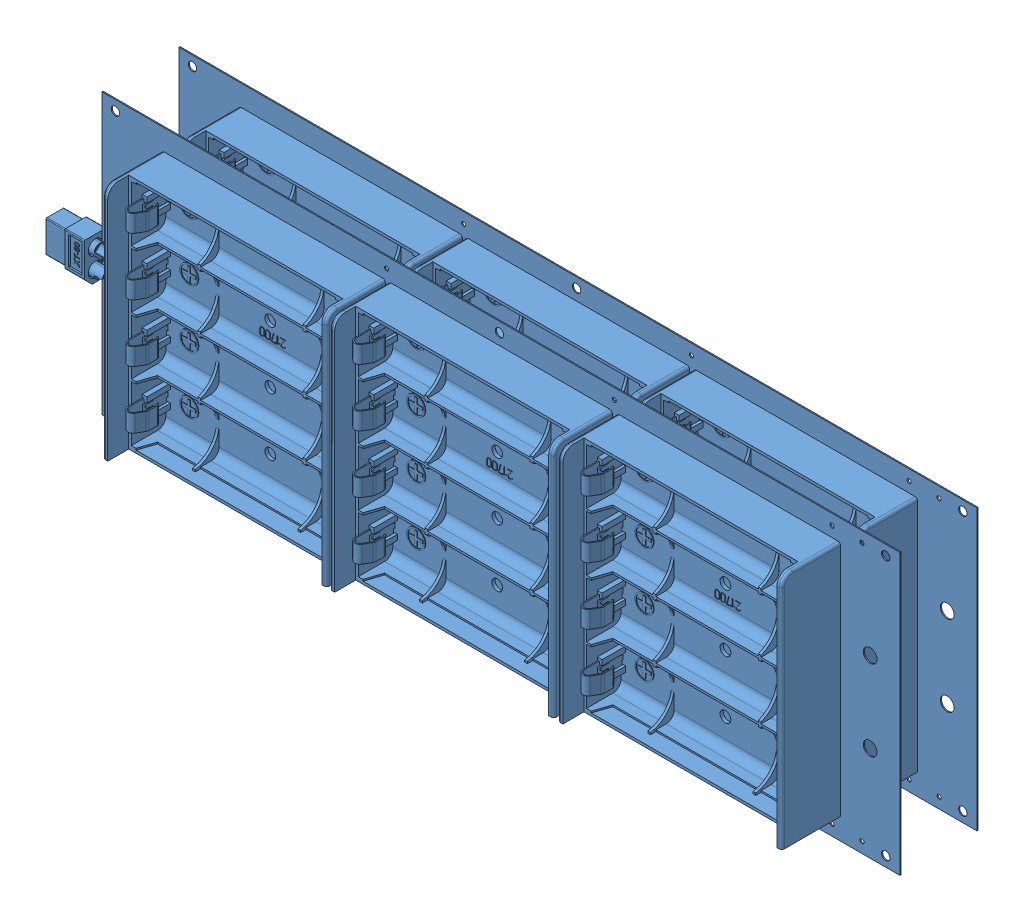
SolidWorks assembly Сборка батареи, configuration Default. Lengths in mm.
Overall size (312.38 103.76 58.38).
2 component instances, 1 part files, 3 mates.
Components (placement in the parent):
- Batarey.step-1: Batarey.step [Default] at origin size (312.38 103.76 29.78)
- Batarey.step-2: Batarey.step [Default] at (0 0 28.6) size (312.38 103.76 29.78)
Mates (geometry in assembly coordinates):
- Coincident1: coincident aligned: plane of Batarey.step-1 through (0 0 0) normal (0 0 1)
- Coincident2: coincident aligned: plane of Batarey.step-1 through (0 0 0) normal (0 1 0)
- Coincident3: coincident aligned: plane of Batarey.step-1 through (0 0 0) normal (1 0 0)
